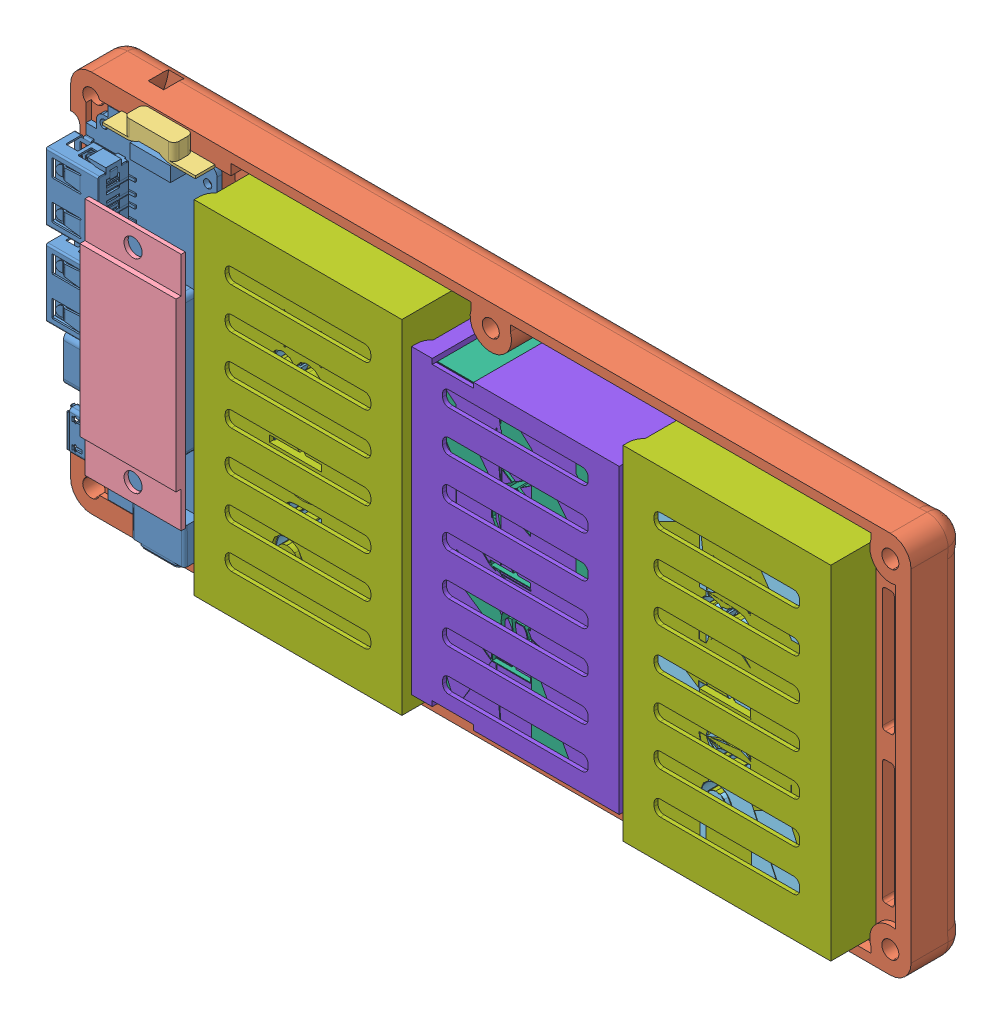
SolidWorks assembly Assem1, configuration По умолчанию. Lengths in mm.
Overall size (162.55 74.06 19.5).
11 component instances, 9 part files, 36 mates.
Components (placement in the parent):
- top-1: top [Default] at (90.9062 111.6947 94.9248) size (162.55 74.06 21) (hidden)
- 1H961_U V6.0.step-1: 1H961_U V6.0.step [Default] at (12.6562 144.6947 104.4248) x (0 -1 0) z (0 0 1) size (68.65 26.68 7.5)
- bottom-1: bottom [По умолчанию] at (90.9062 111.6947 94.9248) size (162.55 74.06 10.5)
- button-1: button [По умолчанию] at (28.919 144.9947 107.6648) x (-1 0 0) z (0 1 0) size (18 3.78 3.7)
- display_glass-1: display_glass [По умолчанию] at (29.7362 111.6947 114.4248) x (0 -1 0) z (0 0 -1) size (46.3 18.6 1.8)
- salt_flat_battery_8x-1: salt_flat_battery_8x [По умолчанию] at (61.5059 79.7568 104.4248) x (-1 0 0) z (0 1 0) size (38 14 64)
- salt_flat_battery_8x-2: salt_flat_battery_8x [По умолчанию] at (143.6307 79.3841 104.4248) x (-1 0 0) z (0 1 0) size (38 14 64)
- salt_flat_battery_7x-1: salt_flat_battery_7x [По умолчанию] at (102.7327 83.6796 104.4248) x (-1 0 0) z (0 1 0) size (38 14 56)
- salt_flat_battery_8x_holder-1: salt_flat_battery_8x_holder [Default] at (61.3559 79.9068 105.2248) x (-1 0 0) z (0 1 0) size (40.15 15.8 66.3)
- salt_flat_battery_8x_holder-2: salt_flat_battery_8x_holder [Default] at (143.4807 79.4341 104.4248) x (-1 0 0) z (0 1 0) size (40.15 15.8 66.3)
- salt_flat_battery_7x_holder-1: salt_flat_battery_7x_holder [Default] at (102.5827 83.5296 104.4248) x (-1 0 0) z (0 1 0) size (40.15 15.8 58.3)
Mates (geometry in assembly coordinates):
- Coincident6: coincident aligned: line of top-1 through (168.1562 148.6947 105.4248) axis (-1 0 0); line of bottom-1 through (168.1562 148.6947 105.4248) axis (-1 0 0)
- Coincident7: coincident aligned: line of top-1 through (13.6562 74.6947 105.4248) axis (1 0 0); line of bottom-1 through (13.6562 74.6947 105.4248) axis (1 0 0)
- Distance3: distance = 0.1 mm anti-aligned: plane of 1H961_U V6.0.step-1 through (36.4562 144.6947 105.4248) normal (0 1 0); plane of bottom-1 through (40.6562 144.7947 128.6594) normal (0 -1 0)
- Coincident14: coincident anti-aligned: plane of 1H961_U V6.0.step-1 through (36.4562 143.1947 104.4248) normal (0 0 -1); plane of bottom-1 through (168.1562 144.6947 104.4248) normal (0 0 1)
- Coincident16: coincident aligned: line of top-1 through (9.6562 83.1947 105.4248) axis (0 -1 0); line of bottom-1 through (9.6562 83.1947 105.4248) axis (0 -1 0)
- Coincident17: coincident aligned: line of 1H961_U V6.0.step-1 through (12.6562 139.6947 105.4248) axis (0 -1 0); line of bottom-1 through (12.6562 143.0823 105.4248) axis (0 -1 0)
- Parallel5: parallel anti-aligned: plane of top-1 through (33.0062 159.514 109.5548) normal (0 0 -1); plane of button-1 through (37.919 145.4947 109.5548) normal (0 0 1)
- Parallel6: parallel anti-aligned: line of top-1 through (19.0062 145.7947 105.4248) axis (1 0 0); line of button-1 through (37.919 144.9947 105.7748) axis (-1 0 0)
- Coincident51: coincident anti-aligned: plane of bottom-1 through (168.1562 144.6947 97.4248) normal (0 0 1); plane of salt_flat_battery_8x-1 through (80.5059 143.7568 97.4248) normal (0 0 -1)
- Coincident58: coincident anti-aligned: plane of bottom-1 through (168.1562 144.6947 97.4248) normal (0 0 1); plane of salt_flat_battery_8x-2 through (162.6307 143.3841 97.4248) normal (0 0 -1)
- Coincident60: coincident anti-aligned: plane of bottom-1 through (168.1562 144.6947 97.4248) normal (0 0 1); plane of salt_flat_battery-9 through (163.4204 132.5061 97.4248) normal (0 0 -1)
- Parallel11: parallel anti-aligned: plane of bottom-1 through (13.6562 77.6947 105.4248) normal (0 1 0); plane of salt_flat_battery-9 through (163.4204 94.5061 111.4248) normal (0 -1 0)
- Coincident62: coincident anti-aligned: plane of bottom-1 through (168.1562 144.6947 97.4248) normal (0 0 1); plane of salt_flat_battery-10 through (171.1758 132.5568 97.4248) normal (0 0 -1)
- Coincident64: coincident aligned: line of salt_flat_battery-9 through (163.4204 94.5061 111.4248) axis (0 0 -1); line of salt_flat_battery-10 through (163.4204 94.5061 111.4248) axis (0 0 -1)
- Coincident69: coincident anti-aligned: plane of bottom-1 through (168.1562 144.6947 97.4248) normal (0 0 1); plane of salt_flat_battery_6x-1 through (121.7327 139.6796 97.4248) normal (0 0 -1)
- Parallel12: parallel aligned: line of salt_flat_battery_8x-1 through (80.5059 143.7568 97.4248) axis (0 -1 0); line of salt_flat_battery_6x-1 through (83.7327 139.6796 97.4248) axis (0 -1 0)
- Coincident71: coincident anti-aligned: plane of bottom-1 through (168.1562 144.6947 97.4248) normal (0 0 1); plane of salt_flat_battery_8x_holder-1 through (61.3559 79.9068 97.4248) normal (0 0 -1)
- Coincident72: coincident anti-aligned: plane of salt_flat_battery_8x-1 through (80.5059 143.7568 97.4248) normal (1 0 0); plane of salt_flat_battery_8x_holder-1 through (80.5059 79.7568 189.9843) normal (-1 0 0)
- Coincident73: coincident anti-aligned: plane of salt_flat_battery_8x-1 through (61.5059 79.7568 104.4248) normal (0 -1 0); plane of salt_flat_battery_8x_holder-1 through (41.3559 79.7568 189.9843) normal (0 1 0)
- Coincident74: coincident anti-aligned: plane of bottom-1 through (168.1562 144.6947 97.4248) normal (0 0 1); plane of salt_flat_battery_8x_holder-1 through (61.3559 79.9068 97.4248) normal (0 0 -1)
- Parallel13: parallel anti-aligned: line of bottom-1 through (40.6562 77.6947 97.4248) axis (1 0 0); line of salt_flat_battery_8x_holder-1 through (81.5059 78.7568 97.4248) axis (-1 0 0)
- Parallel15: parallel anti-aligned: plane of salt_flat_battery_8x-2 through (162.6307 143.3841 97.4248) normal (0 0 -1); plane of salt_flat_battery_8x_holder-2 through (143.4807 79.4341 97.4248) normal (0 0 1)
- Coincident80: coincident anti-aligned: plane of salt_flat_battery_8x-2 through (162.6307 143.3841 97.4248) normal (1 0 0); plane of salt_flat_battery_8x_holder-2 through (162.6307 79.2841 189.1843) normal (-1 0 0)
- Coincident82: coincident anti-aligned: plane of salt_flat_battery_8x-2 through (162.6307 143.3841 97.4248) normal (0 0 -1); plane of salt_flat_battery_8x_holder-2 through (143.4807 79.4341 97.4248) normal (0 0 1)
- Distance4: distance = 0.2 mm anti-aligned: plane of salt_flat_battery_8x-2 through (143.6307 143.3841 104.4248) normal (0 1 0); plane of salt_flat_battery_8x_holder-2 through (162.6307 143.5841 189.1843) normal (0 -1 0)
- Parallel16: parallel anti-aligned: plane of bottom-1 through (168.1562 144.6947 97.4248) normal (0 0 1); plane of salt_flat_battery_8x_holder-2 through (143.4807 79.4341 96.6248) normal (0 0 -1)
- Coincident85: coincident anti-aligned: plane of salt_flat_battery_7x-1 through (121.7327 139.6796 97.4248) normal (0 0 -1); plane of salt_flat_battery_7x_holder-1 through (102.5827 83.5296 97.4248) normal (0 0 1)
- Parallel17: parallel anti-aligned: line of salt_flat_battery_7x-1 through (121.7327 83.6796 97.4248) axis (-1 0 0); line of salt_flat_battery_7x_holder-1 through (82.5827 82.3796 97.4248) axis (1 0 0)
- Coincident87: coincident anti-aligned: plane of salt_flat_battery_7x-1 through (121.7327 139.6796 97.4248) normal (1 0 0); plane of salt_flat_battery_7x_holder-1 through (121.7327 139.6796 182.4626) normal (-1 0 0)
- Parallel18: parallel anti-aligned: plane of bottom-1 through (168.1562 144.6947 97.4248) normal (0 0 1); plane of salt_flat_battery_7x_holder-1 through (102.5827 83.5296 96.6248) normal (0 0 -1)
- Coincident89: coincident anti-aligned: plane of salt_flat_battery_7x-1 through (102.7327 139.6796 104.4248) normal (0 1 0); plane of salt_flat_battery_7x_holder-1 through (82.5827 139.6796 182.4626) normal (0 -1 0)
- Coincident95: coincident aligned: plane of top-1 through (90.9062 148.6947 113.4248) normal (0 1 0); plane of button-1 through (25.094 148.6947 106.7748) normal (0 1 0)
- Concentric1: concentric aligned: circle of top-1; circle of display_glass-1
- Concentric2: concentric aligned: circle of top-1; circle of display_glass-1
- Coincident96: coincident anti-aligned: plane of top-1 through (90.9062 111.6947 114.4248) normal (0 0 -1); plane of display_glass-1 through (29.7362 111.6947 114.4248) normal (0 0 1)
- Coincident97: coincident anti-aligned: plane of top-1 through (33.0062 159.514 109.5548) normal (0 0 -1); plane of button-1 through (37.919 145.4947 109.5548) normal (0 0 1)
